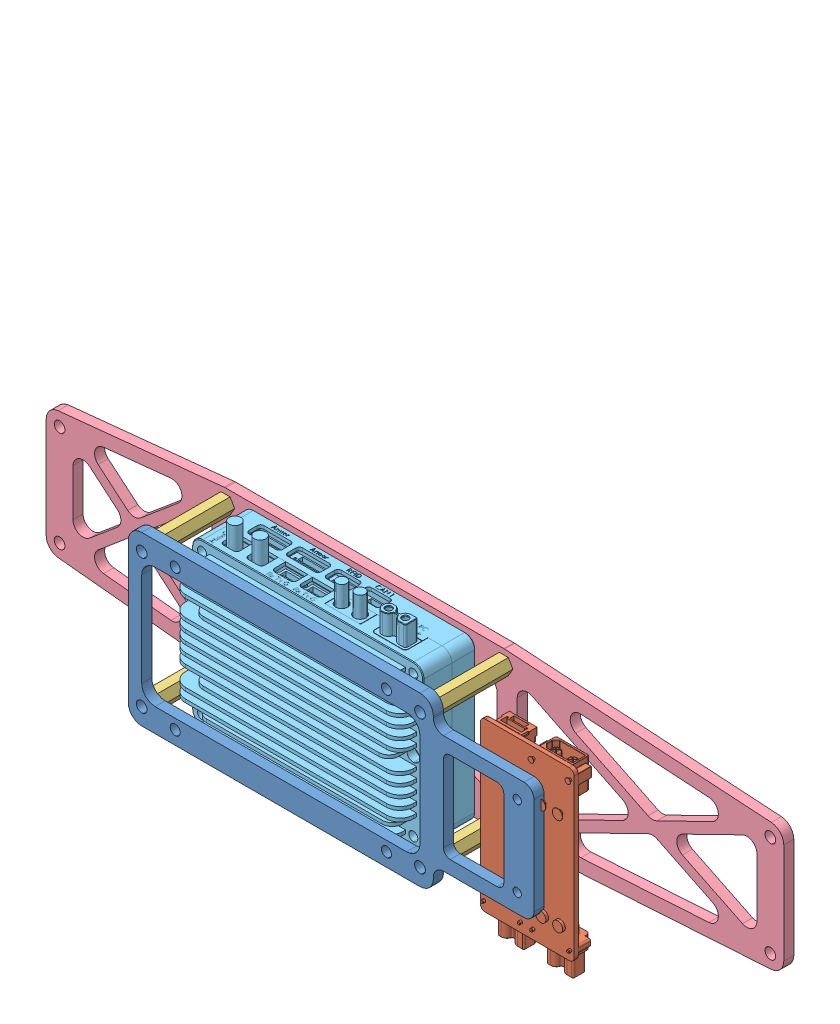
SolidWorks assembly 电管电容, configuration 默认. Lengths in mm.
Overall size (220 198.5 28).
8 component instances, 5 part files, 18 mates.
Components (placement in the parent):
- DP_电容管理模块安装板_1-1: DP_电容管理模块安装板_1 [默认] at origin size (121 50 3)
- DP_RoboMaster 超级电容管理模块 CM01-1: DP_RoboMaster 超级电容管理模块 CM01 [默认] at (70.5 0 -0.6) x (0 -1 0) z (1 0 0) size (56 7.26 28)
- DP_铝柱_M3x22-1: DP_铝柱_M3x22 [默认] at (41.5 -20 -11) size (5.43 4.7 22)
- DP_铝柱_M3x22-2: DP_铝柱_M3x22 [默认] at (-41.5 20 -11) size (5.43 4.7 22)
- DP_铝柱_M3x22-3: DP_铝柱_M3x22 [默认] at (41.5 20 -11) size (5.43 4.7 22)
- DP_铝柱_M3x22-4: DP_铝柱_M3x22 [默认] at (-41.5 -20 -11) size (5.43 4.7 22)
- 电管电容安放版-1: 电管电容安放版 [默认] at (15 0 -25) size (220 48 3)
- DP_RoboMaster 电源模块 PM02 2020-2: DP_RoboMaster 电源模块 PM02 2020 [默认] at (-35.5843 22.8772 -14.2071) x (1 0 0) z (0 1 0) size (70.01 22.52 197.96)
Mates (geometry in assembly coordinates):
- 重合2: coincident anti-aligned: plane of DP_电容管理模块安装板_1-1 through (0 0 0) normal (0 0 -1); plane of DP_RoboMaster 超级电容管理模块 CM01-1 through (70.5 0 0) normal (0 0 1)
- 同心3: concentric aligned: cylinder of DP_电容管理模块安装板_1-1 through (70.5 12 10) axis (0 0 -1) radius 1.25; cylinder of DP_RoboMaster 超级电容管理模块 CM01-1 through (70.5 12 -1.2) axis (0 0 -1) radius 1.1
- 同心4: concentric aligned: cylinder of DP_电容管理模块安装板_1-1 through (70.5 -12 10) axis (0 0 -1) radius 1.25; cylinder of DP_RoboMaster 超级电容管理模块 CM01-1 through (70.5 -12 -1.2) axis (0 0 -1) radius 1.1
- 重合3: coincident anti-aligned: plane of DP_电容管理模块安装板_1-1 through (0 0 0) normal (0 0 -1); plane of DP_铝柱_M3x22-1 through (41.5 -20 0) normal (0 0 1)
- 重合4: coincident aligned: plane of DP_铝柱_M3x22-2 through (-41.5 20 0) normal (0 0 1); plane of DP_铝柱_M3x22-3 through (41.5 20 0) normal (0 0 1)
- 重合5: coincident aligned: plane of DP_铝柱_M3x22-3 through (41.5 20 0) normal (0 0 1); plane of DP_铝柱_M3x22-4 through (-41.5 -20 0) normal (0 0 1)
- 重合6: coincident anti-aligned: plane of DP_电容管理模块安装板_1-1 through (0 0 0) normal (0 0 -1); plane of DP_铝柱_M3x22-3 through (41.5 20 0) normal (0 0 1)
- 同心8: concentric aligned: cylinder of DP_电容管理模块安装板_1-1 through (-41.5 -20 0) axis (0 0 1) radius 1.6; cylinder of DP_铝柱_M3x22-4 through (-41.5 -20 0) axis (0 0 1) radius 1.25
- 同心9: concentric aligned: cylinder of DP_电容管理模块安装板_1-1 through (-41.5 20 0) axis (0 0 1) radius 1.6; cylinder of DP_铝柱_M3x22-2 through (-41.5 20 0) axis (0 0 1) radius 1.25
- 同心10: concentric aligned: cylinder of DP_电容管理模块安装板_1-1 through (41.5 20 0) axis (0 0 1) radius 1.6; cylinder of DP_铝柱_M3x22-3 through (41.5 20 0) axis (0 0 1) radius 1.25
- 同心11: concentric aligned: cylinder of DP_电容管理模块安装板_1-1 through (41.5 -20 0) axis (0 0 1) radius 1.6; cylinder of DP_铝柱_M3x22-1 through (41.5 -20 0) axis (0 0 1) radius 1.25
- 重合7: coincident anti-aligned: plane of DP_铝柱_M3x22-4 through (-41.5 -20 -22) normal (0 0 -1); plane of 电管电容安放版-1 through (15 0 -22) normal (0 0 1)
- 同心12: concentric anti-aligned: cylinder of DP_铝柱_M3x22-4 through (-41.5 -20 0) axis (0 0 1) radius 1.25; cylinder of 电管电容安放版-1 through (-41.5 -20 -22) axis (0 0 -1) radius 1.6
- 同心13: concentric anti-aligned: cylinder of DP_铝柱_M3x22-2 through (-41.5 20 0) axis (0 0 1) radius 1.25; cylinder of 电管电容安放版-1 through (-41.5 20 -22) axis (0 0 -1) radius 1.6
- 同心14: concentric aligned: cylinder of DP_铝柱_M3x22-1 through (41.5 -20 0) axis (0 0 1) radius 1.25; circle of 电管电容安放版-1
- 同心15: concentric: cylinder of DP_电容管理模块安装板_1-1 through (31.5 21 0) axis (0 0 1) radius 1.5; cylinder of DP_RoboMaster 电源模块 PM02 2020-2 through (31.5 21 -9.5) axis (0 0 -1) radius 1.35
- 同心16: concentric: cylinder of DP_电容管理模块安装板_1-1 through (-31.5 21 0) axis (0 0 1) radius 1.5; cylinder of DP_RoboMaster 电源模块 PM02 2020-2 through (-31.5 21 -9.5) axis (0 0 -1) radius 1.35
- 重合8: coincident: plane of DP_电容管理模块安装板_1-1 through (0 0 0) normal (0 0 -1); line of DP_RoboMaster 电源模块 PM02 2020-2 through (28.5 -15.5 0) axis (-1 0 0)
